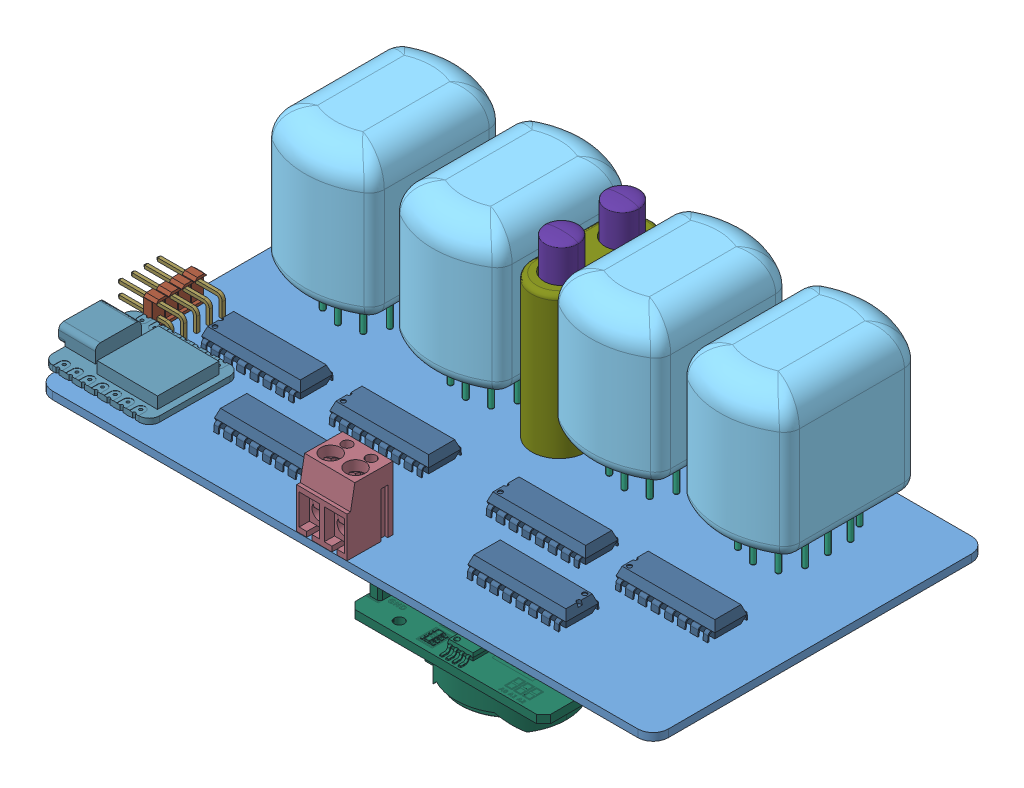
SolidWorks assembly nixie-display, configuration Défaut. Lengths in mm.
Overall size (127.16 50.53 67.27).
292 component instances, 54 part files, 24 mates.
Components (placement in the parent):
- pcb-1: pcb [Défaut] at origin size (121.6 1.5 65.9)
- IN-12A.stp-1: IN-12A.stp [Défaut] at (-40.9487 32.5 -15.5981) x (0 1 0) z (1 0 0) size (35 31 21)
  - 2.stp-1: 2.stp [Défaut] at origin size (2.7 24.17 15.83)
  - 3.stp-1: 3.stp [Défaut] at (-12.2 0 0) x (0 0 -1) z (-1 0 0) size (2 1.5 18.5)
  - 4.stp-1: 4.stp [Défaut] at (-12.2 0 0) x (0 0 1) z (-1 0 0) size (2 1.5 18.5)
  - 5.stp-1: 5.stp [Défaut] at (-12 0 0) x (0 0 -1) z (1 0 0) size (2.1 2.1 1)
  - 5.stp-2: 5.stp [Défaut] at (-10.8 0 0) x (0 0 -1) z (1 0 0) size (2.1 2.1 1)
  - 5.stp-3: 5.stp [Défaut] at (-9.6 0 0) x (0 0 -1) z (1 0 0) size (2.1 2.1 1)
  - 5.stp-4: 5.stp [Défaut] at (-8.4 0 0) x (0 0 -1) z (1 0 0) size (2.1 2.1 1)
  - 5.stp-5: 5.stp [Défaut] at (-7.2 0 0) x (0 0 -1) z (1 0 0) size (2.1 2.1 1)
  - 5.stp-6: 5.stp [Défaut] at (-6 0 0) x (0 0 -1) z (1 0 0) size (2.1 2.1 1)
  - 5.stp-7: 5.stp [Défaut] at (-4.8 0 0) x (0 0 -1) z (1 0 0) size (2.1 2.1 1)
  - 5.stp-8: 5.stp [Défaut] at (-3.6 0 0) x (0 0 -1) z (1 0 0) size (2.1 2.1 1)
  - 5.stp-9: 5.stp [Défaut] at (-2.4 0 0) x (0 0 -1) z (1 0 0) size (2.1 2.1 1)
  - 5.stp-10: 5.stp [Défaut] at (-1.2 0 0) x (0 0 -1) z (1 0 0) size (2.1 2.1 1)
  - 6.stp-1: 6.stp [Défaut] at (-11 16.1596 7.8778) x (0 -0.787778 0.61596) z (-1 0 0) size (2.1 2.1 1)
  - 7.stp-1: 7.stp [Défaut] at (-9.8 16.1596 7.8778) x (0 -0.787778 0.61596) z (-1 0 0) size (2.1 2.1 1)
  - 8.stp-1: 8.stp [Défaut] at (-8.6 16.1596 7.8778) x (0 -0.787778 0.61596) z (-1 0 0) size (2.1 2.1 1)
  - 9.stp-1: 9.stp [Défaut] at (-7.4 16.1596 7.8778) x (0 -0.787778 0.61596) z (-1 0 0) size (2.1 2.1 1)
  - 10.stp-1: 10.stp [Défaut] at (-6.2 16.1596 7.8778) x (0 -0.787778 0.61596) z (-1 0 0) size (2.1 2.1 1)
  - 11.stp-1: 11.stp [Défaut] at (-5 16.1596 7.8778) x (0 -0.787778 0.61596) z (-1 0 0) size (2.1 2.1 1)
  - 12.stp-1: 12.stp [Défaut] at (-3.8 16.1596 7.8778) x (0 -0.787778 0.61596) z (-1 0 0) size (2.1 2.1 1)
  - 13.stp-1: 13.stp [Défaut] at (-2.6 16.1596 7.8778) x (0 -0.787778 0.61596) z (-1 0 0) size (2.1 2.1 1)
  - 14.stp-1: 14.stp [Défaut] at (-1.4 16.1596 7.8778) x (0 -0.787778 0.61596) z (-1 0 0) size (2.1 2.1 1)
  - 15.stp-1: 15.stp [Défaut] at (-0.2 16.1596 7.8778) x (0 -0.787778 0.61596) z (-1 0 0) size (2.1 2.1 1)
  - 5.stp-11: 5.stp [Défaut] x (0 0 -1) z (1 0 0) size (2.1 2.1 1)
  - 5.stp-12: 5.stp [Défaut] at (-13.2 0 0) x (0 0 -1) z (1 0 0) size (2.1 2.1 1)
  - 16.stp-1: 16.stp [Défaut] at (1 16.1596 7.8778) x (0 -0.787778 0.61596) z (-1 0 0) size (2.1 2.1 1)
  - 17.stp-1: 17.stp [Défaut] at (-12.2 16.1596 7.8778) x (0 -0.787778 0.61596) z (-1 0 0) size (2.1 2.1 1)
  - 18.stp-1: 18.stp [Défaut] at (-13.2 0 0) x (0 0 -1) z (-1 0 0) size (15.83 24.17 12.28)
  - 19.stp-1: 19.stp [Défaut] x (1 0 0) z (0 1 0) size (1.51 1.46 20.68)
  - 20.stp-1: 20.stp [Défaut] at (1 0 0) size (4 22.27 2.42)
  - 21.stp-1: 21.stp [Défaut] at (-13.4 0 0) x (0 0 -1) z (-1 0 0) size (15.83 24.17 1)
  - 22.stp-1: 22.stp [Défaut] at (-14.4 0 0) x (0 0 -1) z (-1 0 0) size (15.83 27.29 2)
  - 23.stp-1: 23.stp [Défaut] x (0 0 -1) z (-1 0 0) size (21 31 33)
  - 24.stp-1: 24.stp [Défaut] x (0 0 -1) z (-1 0 0) size (1 1 15.5)
  - 24.stp-2: 24.stp [Défaut] at (0 -4.5 0) x (0 0 -1) z (-1 0 0) size (1 1 15.5)
  - 24.stp-3: 24.stp [Défaut] at (0 -8 -1.75) x (0 0 -1) z (-1 0 0) size (1 1 15.5)
  - 24.stp-4: 24.stp [Défaut] at (0 -9 -5.75) x (0 0 -1) z (-1 0 0) size (1 1 15.5)
  - 24.stp-5: 24.stp [Défaut] at (0 -8 -9.75) x (0 0 -1) z (-1 0 0) size (1 1 15.5)
  - 24.stp-6: 24.stp [Défaut] at (0 -4.5 -11.5) x (0 0 -1) z (-1 0 0) size (1 1 15.5)
  - 24.stp-7: 24.stp [Défaut] at (0 0 -11.5) x (0 0 -1) z (-1 0 0) size (1 1 15.5)
  - 24.stp-8: 24.stp [Défaut] at (0 4.5 -11.5) x (0 0 -1) z (-1 0 0) size (1 1 15.5)
  - 24.stp-9: 24.stp [Défaut] at (0 8 -9.75) x (0 0 -1) z (-1 0 0) size (1 1 15.5)
  - 24.stp-10: 24.stp [Défaut] at (0 9 -5.75) x (0 0 -1) z (-1 0 0) size (1 1 15.5)
  - 24.stp-11: 24.stp [Défaut] at (0 8 -1.75) x (0 0 -1) z (-1 0 0) size (1 1 15.5)
  - 24.stp-12: 24.stp [Défaut] at (0 4.5 0) x (0 0 -1) z (-1 0 0) size (1 1 15.5)
  - 25.stp-1: 25.stp [Défaut] at (-1.4 0 0) x (0 0 1) z (1 0 0) size (10.55 22 0.2)
  - 26.stp-1: 26.stp [Défaut] at (-2.6 0 0) x (0 0 1) z (1 0 0) size (11 22 0.2)
  - 27.stp-1: 27.stp [Défaut] at (-3.8 0 0) x (0 0 1) z (1 0 0) size (11 22 0.2)
  - 28.stp-1: 28.stp [Défaut] at (-5 0 0) x (0 0 1) z (1 0 0) size (10 22 0.2)
  - 29.stp-1: 29.stp [Défaut] at (-7.4 0 0) x (0 0 1) z (1 0 0) size (10 22 0.2)
  - 30.stp-1: 30.stp [Défaut] at (-9.6 0 0) x (0 0 -1) z (-1 0 0) size (10 22 0.2)
  - 31.stp-1: 31.stp [Défaut] at (-11 0 0) x (0 0 1) z (1 0 0) size (11 22 0.2)
  - 32.stp-1: 32.stp [Défaut] at (-12.2 0 0) x (0 0 1) z (1 0 0) size (2 22 0.2)
  - 33.stp-1: 33.stp [Défaut] at (-6 0 0) x (0 0 -1) z (-1 0 0) size (11 22 0.2)
  - 34.stp-1: 34.stp [Défaut] at (-8.6 0 0) x (0 0 1) z (1 0 0) size (10 22 0.2)
  - 1.stp-1: 1.stp [Défaut] at origin size (7.54 3.19 3.19)
  - 1-0.stp-1: 1-0.stp [Défaut] at origin size (11.99 9.11 6.32)
  - 1-1.stp-1: 1-1.stp [Défaut] at origin size (5.03 4.26 4.61)
  - 1-2.stp-1: 1-2.stp [Défaut] at origin size (8.17 8.42 6.65)
  - 1-3.stp-1: 1-3.stp [Défaut] at origin size (17.22 12.89 7.69)
  - 1-4.stp-1: 1-4.stp [Défaut] at origin size (13.11 12.81 7.39)
  - 1-5.stp-1: 1-5.stp [Défaut] at origin size (15.91 7.54 6.9)
  - 1-6.stp-1: 1-6.stp [Défaut] at origin size (10.39 4.47 4.23)
  - 1-7.stp-1: 1-7.stp [Défaut] at origin size (7.32 4.98 2.44)
  - 1-8.stp-1: 1-8.stp [Défaut] at origin size (10.29 4.36 5.63)
  - 1-9.stp-1: 1-9.stp [Défaut] at origin size (12.89 8.1 7.83)
- IN-12A.stp-2: IN-12A.stp [Défaut] at (15.5408 32.5 -15.6508) x (0 1 0) z (1 0 0) size (35 31 21)
  - 2.stp-1: 2.stp [Défaut] at origin size (2.7 24.17 15.83)
  - 3.stp-1: 3.stp [Défaut] at (-12.2 0 0) x (0 0 -1) z (-1 0 0) size (2 1.5 18.5)
  - 4.stp-1: 4.stp [Défaut] at (-12.2 0 0) x (0 0 1) z (-1 0 0) size (2 1.5 18.5)
  - 5.stp-1: 5.stp [Défaut] at (-12 0 0) x (0 0 -1) z (1 0 0) size (2.1 2.1 1)
  - 5.stp-2: 5.stp [Défaut] at (-10.8 0 0) x (0 0 -1) z (1 0 0) size (2.1 2.1 1)
  - 5.stp-3: 5.stp [Défaut] at (-9.6 0 0) x (0 0 -1) z (1 0 0) size (2.1 2.1 1)
  - 5.stp-4: 5.stp [Défaut] at (-8.4 0 0) x (0 0 -1) z (1 0 0) size (2.1 2.1 1)
  - 5.stp-5: 5.stp [Défaut] at (-7.2 0 0) x (0 0 -1) z (1 0 0) size (2.1 2.1 1)
  - 5.stp-6: 5.stp [Défaut] at (-6 0 0) x (0 0 -1) z (1 0 0) size (2.1 2.1 1)
  - 5.stp-7: 5.stp [Défaut] at (-4.8 0 0) x (0 0 -1) z (1 0 0) size (2.1 2.1 1)
  - 5.stp-8: 5.stp [Défaut] at (-3.6 0 0) x (0 0 -1) z (1 0 0) size (2.1 2.1 1)
  - 5.stp-9: 5.stp [Défaut] at (-2.4 0 0) x (0 0 -1) z (1 0 0) size (2.1 2.1 1)
  - 5.stp-10: 5.stp [Défaut] at (-1.2 0 0) x (0 0 -1) z (1 0 0) size (2.1 2.1 1)
  - 6.stp-1: 6.stp [Défaut] at (-11 16.1596 7.8778) x (0 -0.787778 0.61596) z (-1 0 0) size (2.1 2.1 1)
  - 7.stp-1: 7.stp [Défaut] at (-9.8 16.1596 7.8778) x (0 -0.787778 0.61596) z (-1 0 0) size (2.1 2.1 1)
  - 8.stp-1: 8.stp [Défaut] at (-8.6 16.1596 7.8778) x (0 -0.787778 0.61596) z (-1 0 0) size (2.1 2.1 1)
  - 9.stp-1: 9.stp [Défaut] at (-7.4 16.1596 7.8778) x (0 -0.787778 0.61596) z (-1 0 0) size (2.1 2.1 1)
  - 10.stp-1: 10.stp [Défaut] at (-6.2 16.1596 7.8778) x (0 -0.787778 0.61596) z (-1 0 0) size (2.1 2.1 1)
  - 11.stp-1: 11.stp [Défaut] at (-5 16.1596 7.8778) x (0 -0.787778 0.61596) z (-1 0 0) size (2.1 2.1 1)
  - 12.stp-1: 12.stp [Défaut] at (-3.8 16.1596 7.8778) x (0 -0.787778 0.61596) z (-1 0 0) size (2.1 2.1 1)
  - 13.stp-1: 13.stp [Défaut] at (-2.6 16.1596 7.8778) x (0 -0.787778 0.61596) z (-1 0 0) size (2.1 2.1 1)
  - 14.stp-1: 14.stp [Défaut] at (-1.4 16.1596 7.8778) x (0 -0.787778 0.61596) z (-1 0 0) size (2.1 2.1 1)
  - 15.stp-1: 15.stp [Défaut] at (-0.2 16.1596 7.8778) x (0 -0.787778 0.61596) z (-1 0 0) size (2.1 2.1 1)
  - 5.stp-11: 5.stp [Défaut] x (0 0 -1) z (1 0 0) size (2.1 2.1 1)
  - 5.stp-12: 5.stp [Défaut] at (-13.2 0 0) x (0 0 -1) z (1 0 0) size (2.1 2.1 1)
  - 16.stp-1: 16.stp [Défaut] at (1 16.1596 7.8778) x (0 -0.787778 0.61596) z (-1 0 0) size (2.1 2.1 1)
  - 17.stp-1: 17.stp [Défaut] at (-12.2 16.1596 7.8778) x (0 -0.787778 0.61596) z (-1 0 0) size (2.1 2.1 1)
  - 18.stp-1: 18.stp [Défaut] at (-13.2 0 0) x (0 0 -1) z (-1 0 0) size (15.83 24.17 12.28)
  - 19.stp-1: 19.stp [Défaut] x (1 0 0) z (0 1 0) size (1.51 1.46 20.68)
  - 20.stp-1: 20.stp [Défaut] at (1 0 0) size (4 22.27 2.42)
  - 21.stp-1: 21.stp [Défaut] at (-13.4 0 0) x (0 0 -1) z (-1 0 0) size (15.83 24.17 1)
  - 22.stp-1: 22.stp [Défaut] at (-14.4 0 0) x (0 0 -1) z (-1 0 0) size (15.83 27.29 2)
  - 23.stp-1: 23.stp [Défaut] x (0 0 -1) z (-1 0 0) size (21 31 33)
  - 24.stp-1: 24.stp [Défaut] x (0 0 -1) z (-1 0 0) size (1 1 15.5)
  - 24.stp-2: 24.stp [Défaut] at (0 -4.5 0) x (0 0 -1) z (-1 0 0) size (1 1 15.5)
  - 24.stp-3: 24.stp [Défaut] at (0 -8 -1.75) x (0 0 -1) z (-1 0 0) size (1 1 15.5)
  - 24.stp-4: 24.stp [Défaut] at (0 -9 -5.75) x (0 0 -1) z (-1 0 0) size (1 1 15.5)
  - 24.stp-5: 24.stp [Défaut] at (0 -8 -9.75) x (0 0 -1) z (-1 0 0) size (1 1 15.5)
  - 24.stp-6: 24.stp [Défaut] at (0 -4.5 -11.5) x (0 0 -1) z (-1 0 0) size (1 1 15.5)
  - 24.stp-7: 24.stp [Défaut] at (0 0 -11.5) x (0 0 -1) z (-1 0 0) size (1 1 15.5)
  - 24.stp-8: 24.stp [Défaut] at (0 4.5 -11.5) x (0 0 -1) z (-1 0 0) size (1 1 15.5)
  - 24.stp-9: 24.stp [Défaut] at (0 8 -9.75) x (0 0 -1) z (-1 0 0) size (1 1 15.5)
  - 24.stp-10: 24.stp [Défaut] at (0 9 -5.75) x (0 0 -1) z (-1 0 0) size (1 1 15.5)
  - 24.stp-11: 24.stp [Défaut] at (0 8 -1.75) x (0 0 -1) z (-1 0 0) size (1 1 15.5)
  - 24.stp-12: 24.stp [Défaut] at (0 4.5 0) x (0 0 -1) z (-1 0 0) size (1 1 15.5)
  - 25.stp-1: 25.stp [Défaut] at (-1.4 0 0) x (0 0 1) z (1 0 0) size (10.55 22 0.2)
  - 26.stp-1: 26.stp [Défaut] at (-2.6 0 0) x (0 0 1) z (1 0 0) size (11 22 0.2)
  - 27.stp-1: 27.stp [Défaut] at (-3.8 0 0) x (0 0 1) z (1 0 0) size (11 22 0.2)
  - 28.stp-1: 28.stp [Défaut] at (-5 0 0) x (0 0 1) z (1 0 0) size (10 22 0.2)
  - 29.stp-1: 29.stp [Défaut] at (-7.4 0 0) x (0 0 1) z (1 0 0) size (10 22 0.2)
  - 30.stp-1: 30.stp [Défaut] at (-9.6 0 0) x (0 0 -1) z (-1 0 0) size (10 22 0.2)
  - 31.stp-1: 31.stp [Défaut] at (-11 0 0) x (0 0 1) z (1 0 0) size (11 22 0.2)
  - 32.stp-1: 32.stp [Défaut] at (-12.2 0 0) x (0 0 1) z (1 0 0) size (2 22 0.2)
  - 33.stp-1: 33.stp [Défaut] at (-6 0 0) x (0 0 -1) z (-1 0 0) size (11 22 0.2)
  - 34.stp-1: 34.stp [Défaut] at (-8.6 0 0) x (0 0 1) z (1 0 0) size (10 22 0.2)
  - 1.stp-1: 1.stp [Défaut] at origin size (7.54 3.19 3.19)
  - 1-0.stp-1: 1-0.stp [Défaut] at origin size (11.99 9.11 6.32)
  - 1-1.stp-1: 1-1.stp [Défaut] at origin size (5.03 4.26 4.61)
  - 1-2.stp-1: 1-2.stp [Défaut] at origin size (8.17 8.42 6.65)
  - 1-3.stp-1: 1-3.stp [Défaut] at origin size (17.22 12.89 7.69)
  - 1-4.stp-1: 1-4.stp [Défaut] at origin size (13.11 12.81 7.39)
  - 1-5.stp-1: 1-5.stp [Défaut] at origin size (15.91 7.54 6.9)
  - 1-6.stp-1: 1-6.stp [Défaut] at origin size (10.39 4.47 4.23)
  - 1-7.stp-1: 1-7.stp [Défaut] at origin size (7.32 4.98 2.44)
  - 1-8.stp-1: 1-8.stp [Défaut] at origin size (10.29 4.36 5.63)
  - 1-9.stp-1: 1-9.stp [Défaut] at origin size (12.89 8.1 7.83)
- IN-12A.stp-3: IN-12A.stp [Défaut] at (-15.577 32.5 -15.4564) x (0 1 0) z (1 0 0) size (35 31 21)
  - 2.stp-1: 2.stp [Défaut] at origin size (2.7 24.17 15.83)
  - 3.stp-1: 3.stp [Défaut] at (-12.2 0 0) x (0 0 -1) z (-1 0 0) size (2 1.5 18.5)
  - 4.stp-1: 4.stp [Défaut] at (-12.2 0 0) x (0 0 1) z (-1 0 0) size (2 1.5 18.5)
  - 5.stp-1: 5.stp [Défaut] at (-12 0 0) x (0 0 -1) z (1 0 0) size (2.1 2.1 1)
  - 5.stp-2: 5.stp [Défaut] at (-10.8 0 0) x (0 0 -1) z (1 0 0) size (2.1 2.1 1)
  - 5.stp-3: 5.stp [Défaut] at (-9.6 0 0) x (0 0 -1) z (1 0 0) size (2.1 2.1 1)
  - 5.stp-4: 5.stp [Défaut] at (-8.4 0 0) x (0 0 -1) z (1 0 0) size (2.1 2.1 1)
  - 5.stp-5: 5.stp [Défaut] at (-7.2 0 0) x (0 0 -1) z (1 0 0) size (2.1 2.1 1)
  - 5.stp-6: 5.stp [Défaut] at (-6 0 0) x (0 0 -1) z (1 0 0) size (2.1 2.1 1)
  - 5.stp-7: 5.stp [Défaut] at (-4.8 0 0) x (0 0 -1) z (1 0 0) size (2.1 2.1 1)
  - 5.stp-8: 5.stp [Défaut] at (-3.6 0 0) x (0 0 -1) z (1 0 0) size (2.1 2.1 1)
  - 5.stp-9: 5.stp [Défaut] at (-2.4 0 0) x (0 0 -1) z (1 0 0) size (2.1 2.1 1)
  - 5.stp-10: 5.stp [Défaut] at (-1.2 0 0) x (0 0 -1) z (1 0 0) size (2.1 2.1 1)
  - 6.stp-1: 6.stp [Défaut] at (-11 16.1596 7.8778) x (0 -0.787778 0.61596) z (-1 0 0) size (2.1 2.1 1)
  - 7.stp-1: 7.stp [Défaut] at (-9.8 16.1596 7.8778) x (0 -0.787778 0.61596) z (-1 0 0) size (2.1 2.1 1)
  - 8.stp-1: 8.stp [Défaut] at (-8.6 16.1596 7.8778) x (0 -0.787778 0.61596) z (-1 0 0) size (2.1 2.1 1)
  - 9.stp-1: 9.stp [Défaut] at (-7.4 16.1596 7.8778) x (0 -0.787778 0.61596) z (-1 0 0) size (2.1 2.1 1)
  - 10.stp-1: 10.stp [Défaut] at (-6.2 16.1596 7.8778) x (0 -0.787778 0.61596) z (-1 0 0) size (2.1 2.1 1)
  - 11.stp-1: 11.stp [Défaut] at (-5 16.1596 7.8778) x (0 -0.787778 0.61596) z (-1 0 0) size (2.1 2.1 1)
  - 12.stp-1: 12.stp [Défaut] at (-3.8 16.1596 7.8778) x (0 -0.787778 0.61596) z (-1 0 0) size (2.1 2.1 1)
  - 13.stp-1: 13.stp [Défaut] at (-2.6 16.1596 7.8778) x (0 -0.787778 0.61596) z (-1 0 0) size (2.1 2.1 1)
  - 14.stp-1: 14.stp [Défaut] at (-1.4 16.1596 7.8778) x (0 -0.787778 0.61596) z (-1 0 0) size (2.1 2.1 1)
  - 15.stp-1: 15.stp [Défaut] at (-0.2 16.1596 7.8778) x (0 -0.787778 0.61596) z (-1 0 0) size (2.1 2.1 1)
  - 5.stp-11: 5.stp [Défaut] x (0 0 -1) z (1 0 0) size (2.1 2.1 1)
  - 5.stp-12: 5.stp [Défaut] at (-13.2 0 0) x (0 0 -1) z (1 0 0) size (2.1 2.1 1)
  - 16.stp-1: 16.stp [Défaut] at (1 16.1596 7.8778) x (0 -0.787778 0.61596) z (-1 0 0) size (2.1 2.1 1)
  - 17.stp-1: 17.stp [Défaut] at (-12.2 16.1596 7.8778) x (0 -0.787778 0.61596) z (-1 0 0) size (2.1 2.1 1)
  - 18.stp-1: 18.stp [Défaut] at (-13.2 0 0) x (0 0 -1) z (-1 0 0) size (15.83 24.17 12.28)
  - 19.stp-1: 19.stp [Défaut] x (1 0 0) z (0 1 0) size (1.51 1.46 20.68)
  - 20.stp-1: 20.stp [Défaut] at (1 0 0) size (4 22.27 2.42)
  - 21.stp-1: 21.stp [Défaut] at (-13.4 0 0) x (0 0 -1) z (-1 0 0) size (15.83 24.17 1)
  - 22.stp-1: 22.stp [Défaut] at (-14.4 0 0) x (0 0 -1) z (-1 0 0) size (15.83 27.29 2)
  - 23.stp-1: 23.stp [Défaut] x (0 0 -1) z (-1 0 0) size (21 31 33)
  - 24.stp-1: 24.stp [Défaut] x (0 0 -1) z (-1 0 0) size (1 1 15.5)
  - 24.stp-2: 24.stp [Défaut] at (0 -4.5 0) x (0 0 -1) z (-1 0 0) size (1 1 15.5)
  - 24.stp-3: 24.stp [Défaut] at (0 -8 -1.75) x (0 0 -1) z (-1 0 0) size (1 1 15.5)
  - 24.stp-4: 24.stp [Défaut] at (0 -9 -5.75) x (0 0 -1) z (-1 0 0) size (1 1 15.5)
  - 24.stp-5: 24.stp [Défaut] at (0 -8 -9.75) x (0 0 -1) z (-1 0 0) size (1 1 15.5)
  - 24.stp-6: 24.stp [Défaut] at (0 -4.5 -11.5) x (0 0 -1) z (-1 0 0) size (1 1 15.5)
  - 24.stp-7: 24.stp [Défaut] at (0 0 -11.5) x (0 0 -1) z (-1 0 0) size (1 1 15.5)
  - 24.stp-8: 24.stp [Défaut] at (0 4.5 -11.5) x (0 0 -1) z (-1 0 0) size (1 1 15.5)
  - 24.stp-9: 24.stp [Défaut] at (0 8 -9.75) x (0 0 -1) z (-1 0 0) size (1 1 15.5)
  - 24.stp-10: 24.stp [Défaut] at (0 9 -5.75) x (0 0 -1) z (-1 0 0) size (1 1 15.5)
  - 24.stp-11: 24.stp [Défaut] at (0 8 -1.75) x (0 0 -1) z (-1 0 0) size (1 1 15.5)
  - 24.stp-12: 24.stp [Défaut] at (0 4.5 0) x (0 0 -1) z (-1 0 0) size (1 1 15.5)
  - 25.stp-1: 25.stp [Défaut] at (-1.4 0 0) x (0 0 1) z (1 0 0) size (10.55 22 0.2)
  - 26.stp-1: 26.stp [Défaut] at (-2.6 0 0) x (0 0 1) z (1 0 0) size (11 22 0.2)
  - 27.stp-1: 27.stp [Défaut] at (-3.8 0 0) x (0 0 1) z (1 0 0) size (11 22 0.2)
  - 28.stp-1: 28.stp [Défaut] at (-5 0 0) x (0 0 1) z (1 0 0) size (10 22 0.2)
  - 29.stp-1: 29.stp [Défaut] at (-7.4 0 0) x (0 0 1) z (1 0 0) size (10 22 0.2)
  - 30.stp-1: 30.stp [Défaut] at (-9.6 0 0) x (0 0 -1) z (-1 0 0) size (10 22 0.2)
  - 31.stp-1: 31.stp [Défaut] at (-11 0 0) x (0 0 1) z (1 0 0) size (11 22 0.2)
  - 32.stp-1: 32.stp [Défaut] at (-12.2 0 0) x (0 0 1) z (1 0 0) size (2 22 0.2)
  - 33.stp-1: 33.stp [Défaut] at (-6 0 0) x (0 0 -1) z (-1 0 0) size (11 22 0.2)
  - 34.stp-1: 34.stp [Défaut] at (-8.6 0 0) x (0 0 1) z (1 0 0) size (10 22 0.2)
  - 1.stp-1: 1.stp [Défaut] at origin size (7.54 3.19 3.19)
  - 1-0.stp-1: 1-0.stp [Défaut] at origin size (11.99 9.11 6.32)
  - 1-1.stp-1: 1-1.stp [Défaut] at origin size (5.03 4.26 4.61)
  - 1-2.stp-1: 1-2.stp [Défaut] at origin size (8.17 8.42 6.65)
  - 1-3.stp-1: 1-3.stp [Défaut] at origin size (17.22 12.89 7.69)
  - 1-4.stp-1: 1-4.stp [Défaut] at origin size (13.11 12.81 7.39)
  - 1-5.stp-1: 1-5.stp [Défaut] at origin size (15.91 7.54 6.9)
  - 1-6.stp-1: 1-6.stp [Défaut] at origin size (10.39 4.47 4.23)
  - 1-7.stp-1: 1-7.stp [Défaut] at origin size (7.32 4.98 2.44)
  - 1-8.stp-1: 1-8.stp [Défaut] at origin size (10.29 4.36 5.63)
  - 1-9.stp-1: 1-9.stp [Défaut] at origin size (12.89 8.1 7.83)
- IN-12A.stp-4: IN-12A.stp [Défaut] at (40.934 32.5 -15.666) x (0 1 0) z (1 0 0) size (35 31 21)
  - 2.stp-1: 2.stp [Défaut] at origin size (2.7 24.17 15.83)
  - 3.stp-1: 3.stp [Défaut] at (-12.2 0 0) x (0 0 -1) z (-1 0 0) size (2 1.5 18.5)
  - 4.stp-1: 4.stp [Défaut] at (-12.2 0 0) x (0 0 1) z (-1 0 0) size (2 1.5 18.5)
  - 5.stp-1: 5.stp [Défaut] at (-12 0 0) x (0 0 -1) z (1 0 0) size (2.1 2.1 1)
  - 5.stp-2: 5.stp [Défaut] at (-10.8 0 0) x (0 0 -1) z (1 0 0) size (2.1 2.1 1)
  - 5.stp-3: 5.stp [Défaut] at (-9.6 0 0) x (0 0 -1) z (1 0 0) size (2.1 2.1 1)
  - 5.stp-4: 5.stp [Défaut] at (-8.4 0 0) x (0 0 -1) z (1 0 0) size (2.1 2.1 1)
  - 5.stp-5: 5.stp [Défaut] at (-7.2 0 0) x (0 0 -1) z (1 0 0) size (2.1 2.1 1)
  - 5.stp-6: 5.stp [Défaut] at (-6 0 0) x (0 0 -1) z (1 0 0) size (2.1 2.1 1)
  - 5.stp-7: 5.stp [Défaut] at (-4.8 0 0) x (0 0 -1) z (1 0 0) size (2.1 2.1 1)
  - 5.stp-8: 5.stp [Défaut] at (-3.6 0 0) x (0 0 -1) z (1 0 0) size (2.1 2.1 1)
  - 5.stp-9: 5.stp [Défaut] at (-2.4 0 0) x (0 0 -1) z (1 0 0) size (2.1 2.1 1)
  - 5.stp-10: 5.stp [Défaut] at (-1.2 0 0) x (0 0 -1) z (1 0 0) size (2.1 2.1 1)
  - 6.stp-1: 6.stp [Défaut] at (-11 16.1596 7.8778) x (0 -0.787778 0.61596) z (-1 0 0) size (2.1 2.1 1)
  - 7.stp-1: 7.stp [Défaut] at (-9.8 16.1596 7.8778) x (0 -0.787778 0.61596) z (-1 0 0) size (2.1 2.1 1)
  - 8.stp-1: 8.stp [Défaut] at (-8.6 16.1596 7.8778) x (0 -0.787778 0.61596) z (-1 0 0) size (2.1 2.1 1)
  - 9.stp-1: 9.stp [Défaut] at (-7.4 16.1596 7.8778) x (0 -0.787778 0.61596) z (-1 0 0) size (2.1 2.1 1)
  - 10.stp-1: 10.stp [Défaut] at (-6.2 16.1596 7.8778) x (0 -0.787778 0.61596) z (-1 0 0) size (2.1 2.1 1)
  - 11.stp-1: 11.stp [Défaut] at (-5 16.1596 7.8778) x (0 -0.787778 0.61596) z (-1 0 0) size (2.1 2.1 1)
  - 12.stp-1: 12.stp [Défaut] at (-3.8 16.1596 7.8778) x (0 -0.787778 0.61596) z (-1 0 0) size (2.1 2.1 1)
  - 13.stp-1: 13.stp [Défaut] at (-2.6 16.1596 7.8778) x (0 -0.787778 0.61596) z (-1 0 0) size (2.1 2.1 1)
  - 14.stp-1: 14.stp [Défaut] at (-1.4 16.1596 7.8778) x (0 -0.787778 0.61596) z (-1 0 0) size (2.1 2.1 1)
  - 15.stp-1: 15.stp [Défaut] at (-0.2 16.1596 7.8778) x (0 -0.787778 0.61596) z (-1 0 0) size (2.1 2.1 1)
  - 5.stp-11: 5.stp [Défaut] x (0 0 -1) z (1 0 0) size (2.1 2.1 1)
  - 5.stp-12: 5.stp [Défaut] at (-13.2 0 0) x (0 0 -1) z (1 0 0) size (2.1 2.1 1)
  - 16.stp-1: 16.stp [Défaut] at (1 16.1596 7.8778) x (0 -0.787778 0.61596) z (-1 0 0) size (2.1 2.1 1)
  - 17.stp-1: 17.stp [Défaut] at (-12.2 16.1596 7.8778) x (0 -0.787778 0.61596) z (-1 0 0) size (2.1 2.1 1)
  - 18.stp-1: 18.stp [Défaut] at (-13.2 0 0) x (0 0 -1) z (-1 0 0) size (15.83 24.17 12.28)
  - 19.stp-1: 19.stp [Défaut] x (1 0 0) z (0 1 0) size (1.51 1.46 20.68)
  - 20.stp-1: 20.stp [Défaut] at (1 0 0) size (4 22.27 2.42)
  - 21.stp-1: 21.stp [Défaut] at (-13.4 0 0) x (0 0 -1) z (-1 0 0) size (15.83 24.17 1)
  - 22.stp-1: 22.stp [Défaut] at (-14.4 0 0) x (0 0 -1) z (-1 0 0) size (15.83 27.29 2)
  - 23.stp-1: 23.stp [Défaut] x (0 0 -1) z (-1 0 0) size (21 31 33)
  - 24.stp-1: 24.stp [Défaut] x (0 0 -1) z (-1 0 0) size (1 1 15.5)
  - 24.stp-2: 24.stp [Défaut] at (0 -4.5 0) x (0 0 -1) z (-1 0 0) size (1 1 15.5)
  - 24.stp-3: 24.stp [Défaut] at (0 -8 -1.75) x (0 0 -1) z (-1 0 0) size (1 1 15.5)
  - 24.stp-4: 24.stp [Défaut] at (0 -9 -5.75) x (0 0 -1) z (-1 0 0) size (1 1 15.5)
  - 24.stp-5: 24.stp [Défaut] at (0 -8 -9.75) x (0 0 -1) z (-1 0 0) size (1 1 15.5)
  - 24.stp-6: 24.stp [Défaut] at (0 -4.5 -11.5) x (0 0 -1) z (-1 0 0) size (1 1 15.5)
  - 24.stp-7: 24.stp [Défaut] at (0 0 -11.5) x (0 0 -1) z (-1 0 0) size (1 1 15.5)
  - 24.stp-8: 24.stp [Défaut] at (0 4.5 -11.5) x (0 0 -1) z (-1 0 0) size (1 1 15.5)
  - 24.stp-9: 24.stp [Défaut] at (0 8 -9.75) x (0 0 -1) z (-1 0 0) size (1 1 15.5)
  - 24.stp-10: 24.stp [Défaut] at (0 9 -5.75) x (0 0 -1) z (-1 0 0) size (1 1 15.5)
  - 24.stp-11: 24.stp [Défaut] at (0 8 -1.75) x (0 0 -1) z (-1 0 0) size (1 1 15.5)
  - 24.stp-12: 24.stp [Défaut] at (0 4.5 0) x (0 0 -1) z (-1 0 0) size (1 1 15.5)
  - 25.stp-1: 25.stp [Défaut] at (-1.4 0 0) x (0 0 1) z (1 0 0) size (10.55 22 0.2)
  - 26.stp-1: 26.stp [Défaut] at (-2.6 0 0) x (0 0 1) z (1 0 0) size (11 22 0.2)
  - 27.stp-1: 27.stp [Défaut] at (-3.8 0 0) x (0 0 1) z (1 0 0) size (11 22 0.2)
  - 28.stp-1: 28.stp [Défaut] at (-5 0 0) x (0 0 1) z (1 0 0) size (10 22 0.2)
  - 29.stp-1: 29.stp [Défaut] at (-7.4 0 0) x (0 0 1) z (1 0 0) size (10 22 0.2)
  - 30.stp-1: 30.stp [Défaut] at (-9.6 0 0) x (0 0 -1) z (-1 0 0) size (10 22 0.2)
  - 31.stp-1: 31.stp [Défaut] at (-11 0 0) x (0 0 1) z (1 0 0) size (11 22 0.2)
  - 32.stp-1: 32.stp [Défaut] at (-12.2 0 0) x (0 0 1) z (1 0 0) size (2 22 0.2)
  - 33.stp-1: 33.stp [Défaut] at (-6 0 0) x (0 0 -1) z (-1 0 0) size (11 22 0.2)
  - 34.stp-1: 34.stp [Défaut] at (-8.6 0 0) x (0 0 1) z (1 0 0) size (10 22 0.2)
  - 1.stp-1: 1.stp [Défaut] at origin size (7.54 3.19 3.19)
  - 1-0.stp-1: 1-0.stp [Défaut] at origin size (11.99 9.11 6.32)
  - 1-1.stp-1: 1-1.stp [Défaut] at origin size (5.03 4.26 4.61)
  - 1-2.stp-1: 1-2.stp [Défaut] at origin size (8.17 8.42 6.65)
  - 1-3.stp-1: 1-3.stp [Défaut] at origin size (17.22 12.89 7.69)
  - 1-4.stp-1: 1-4.stp [Défaut] at origin size (13.11 12.81 7.39)
  - 1-5.stp-1: 1-5.stp [Défaut] at origin size (15.91 7.54 6.9)
  - 1-6.stp-1: 1-6.stp [Défaut] at origin size (10.39 4.47 4.23)
  - 1-7.stp-1: 1-7.stp [Défaut] at origin size (7.32 4.98 2.44)
  - 1-8.stp-1: 1-8.stp [Défaut] at origin size (10.29 4.36 5.63)
  - 1-9.stp-1: 1-9.stp [Défaut] at origin size (12.89 8.1 7.83)
- DIP18N.step-1: DIP18N.step [Défaut] at (-50.7835 3.7087 35.4382) x (0 0 1) z (-1 0 0) size (8.53 6.85 19.5)
- DIP18N.step-2: DIP18N.step [Défaut] at (31.1067 3.7087 35.4997) x (0 0 1) z (-1 0 0) size (8.53 6.85 19.5)
- DIP18N.step-3: DIP18N.step [Défaut] at (5.6608 3.7087 35.5611) x (0 0 1) z (-1 0 0) size (8.53 6.85 19.5)
- DIP18N.step-4: DIP18N.step [Défaut] at (-25.3559 3.7087 35.5399) x (0 0 1) z (-1 0 0) size (8.53 6.85 19.5)
- DS1022-2x4RF11.stp-1: DS1022-2x4RF11.stp [Défaut] at (-56.1796 1.5 3.5604) x (0 0 1) z (0 1 0) size (10.16 13.04 8)
  - eBom-prt0.stp-1: eBom-prt0.stp [Défaut] at origin size (10.16 2.5 5)
  - eBom-prt1.stp-1: eBom-prt1.stp [Défaut] at origin size (0.64 13.04 7.09)
  - eBom-prt1.stp-2: eBom-prt1.stp [Défaut] at (2.54 0 0) size (0.64 13.04 7.09)
  - eBom-prt1.stp-3: eBom-prt1.stp [Défaut] at (5.08 0 0) size (0.64 13.04 7.09)
  - eBom-prt1.stp-4: eBom-prt1.stp [Défaut] at (7.62 0 0) size (0.64 13.04 7.09)
- DIP18N.step-5: DIP18N.step [Défaut] at (-15.751 3.7087 -7.8923) x (0.008727 0 -0.999962) z (0.999962 0 0.008727) size (8.53 6.85 19.5)
- DIP18N.step-6: DIP18N.step [Défaut] at (34.3108 3.7087 -7.8662) x (0.008727 0 -0.999962) z (0.999962 0 0.008727) size (8.53 6.85 19.5)
- Screw Terminal Block 5mm-2: Screw Terminal Block 5mm [Valor predeterminado] at (0.4217 1.5 23.933) x (-0.999962 0 -0.008727) z (0.008727 0 -0.999962) size (10.6 16.9 9)
- Seeeduino Xiao.step-1: Seeeduino Xiao.step [Défaut] at (-88.5187 11.44 25.9289) x (-0.008727 0 0.999962) z (-0.999962 0 -0.008727) size (17.8 4.27 22.5)
- DS3231 RTC.step-1: DS3231 RTC.step [Défaut] at (21.2627 -4.62 22.922) x (1 0 0) z (0 1 0) size (44.75 22.8 13.53)
- indics-1: indics [Défaut] at (0 1.5 -21.8057) size (10.8 43.17 23.8)
  - indic-holder-1: indic-holder [Défaut] at (0 0 6) size (10.8 28.02 23.8)
  - INS1.STEP-1: INS1.STEP [Défaut] at (0 17 0) x (0 0 1) z (-1 0 0) size (7.01 43.17 6.51)
    - INS1-Glask_rper_01.STEP-1: INS1-Glask_rper_01.STEP [Défaut] at origin size (7.01 28.6 6.51)
    - INS1_Inlay_01.STEP-1: INS1_Inlay_01.STEP [Défaut] at (0 5.1 0) size (6 41.77 5.25)
  - INS1.STEP-2: INS1.STEP [Défaut] at (0 17 12) x (0 0 1) z (-1 0 0) size (7.01 43.17 6.51)
    - INS1-Glask_rper_01.STEP-1: INS1-Glask_rper_01.STEP [Défaut] at origin size (7.01 28.6 6.51)
    - INS1_Inlay_01.STEP-1: INS1_Inlay_01.STEP [Défaut] at (0 5.1 0) size (6 41.77 5.25)
Mates (geometry in assembly coordinates):
- Coïncidente5: coincident anti-aligned: plane of pcb-1 through (0 1.5 0) normal (0 1 0); plane of IN-12A.stp-1/24.stp-8 through (-52.4487 1.5 -11.0981) normal (0 -1 0)
- Parallèle3: parallel aligned: plane of pcb-1 through (-60.8 1.5 -32.95) normal (-1 0 0); plane of IN-12A.stp-1/23.stp-1 through (-51.4487 36.5 -5.24) normal (-1 0 0)
- Coïncidente7: coincident anti-aligned: plane of pcb-1 through (0 1.5 0) normal (0 1 0); plane of IN-12A.stp-3/24.stp-2 through (-15.577 1.5 -19.9564) normal (0 -1 0)
- Coïncidente9: coincident anti-aligned: plane of pcb-1 through (0 1.5 0) normal (0 1 0); plane of IN-12A.stp-4/24.stp-10 through (35.184 1.5 -6.666) normal (0 -1 0)
- Parallèle5: parallel aligned: plane of IN-12A.stp-1/23.stp-1 through (-51.4487 36.5 -5.24) normal (-1 0 0); plane of IN-12A.stp-4/23.stp-1 through (30.434 36.5 -5.308) normal (-1 0 0)
- Coïncidente11: coincident anti-aligned: plane of pcb-1 through (0 1.5 0) normal (0 1 0); circle of IN-12A.stp-2/24.stp-6
- Parallèle6: parallel aligned: plane of IN-12A.stp-1/23.stp-1 through (-51.4487 36.5 -5.24) normal (-1 0 0); plane of IN-12A.stp-2/23.stp-1 through (5.0408 36.5 -5.2927) normal (-1 0 0)
- Coïncidente15: coincident anti-aligned: plane of pcb-1 through (0 1.5 0) normal (0 1 0); plane of DIP18N.step-1 through (-31.2835 1.5 4.7548) normal (0 -1 0)
- Coïncidente16: coincident anti-aligned: plane of pcb-1 through (0 1.5 0) normal (0 1 0); plane of DIP18N.step-4 through (-5.8559 1.5 4.8565) normal (0 -1 0)
- Coïncidente17: coincident anti-aligned: plane of pcb-1 through (0 1.5 0) normal (0 1 0); plane of DIP18N.step-3 through (25.1608 1.5 4.8776) normal (0 -1 0)
- Coïncidente18: coincident anti-aligned: plane of pcb-1 through (0 1.5 0) normal (0 1 0); plane of DIP18N.step-2 through (50.6067 1.5 4.8163) normal (0 -1 0)
- Coïncidente19: coincident anti-aligned: plane of pcb-1 through (0 1.5 0) normal (0 1 0); plane of DS1022-2x4RF11.stp-1/eBom-prt0.stp-1 through (-60.3596 1.5 4.2457) normal (0 -1 0)
- Parallèle7: parallel aligned: plane of pcb-1 through (-60.8 1.5 -32.95) normal (-1 0 0); plane of DS1022-2x4RF11.stp-1/eBom-prt0.stp-1 through (-60.3596 1.5 3.5604) normal (-1 0 0)
- Coïncidente21: coincident anti-aligned: plane of pcb-1 through (0 1.5 0) normal (0 1 0); plane of DIP18N.step-5 through (-35.5181 1.5 22.6198) normal (0 -1 0)
- Coïncidente22: coincident anti-aligned: plane of pcb-1 through (0 1.5 0) normal (0 1 0); plane of DIP18N.step-6 through (14.5438 1.5 22.6458) normal (0 -1 0)
- Coïncidente23: coincident anti-aligned: plane of pcb-1 through (0 1.5 0) normal (0 1 0); plane of Screw Terminal Block 5mm-2 through (-9.6565 1.5 32.8454) normal (0 -1 0)
- Distance1: distance = 2.5 mm anti-aligned: plane of Seeeduino Xiao.step-1 through (-49.894 4 23.2659) normal (0 -1 0); plane of pcb-1 through (0 1.5 0) normal (0 1 0)
- Coïncidente26: coincident aligned: plane of pcb-1 through (0 0 0) normal (1 0 0)
- Coïncidente27: coincident aligned: plane of pcb-1 through (0 0 0) normal (0 0 1)
- Coïncidente28: coincident aligned: plane of pcb-1 through (0 0 0) normal (0 1 0)
- Parallèle8: parallel anti-aligned: plane of pcb-1 through (0 0 0) normal (0 -1 0); plane of DS3231 RTC.step-1 through (21.2627 -4.62 22.922) normal (0 1 0)
- Distance2: distance = 4.62 mm anti-aligned: plane of pcb-1 through (0 0 0) normal (0 -1 0); plane of DS3231 RTC.step-1 through (21.2627 -4.62 22.922) normal (0 1 0)
- Coïncidente29: coincident anti-aligned: plane of pcb-1 through (0 1.5 0) normal (0 1 0); plane of indics-1/indic-holder-1 through (0 1.5 -22.3057) normal (0 -1 0)
- Coïncidente30: coincident aligned: plane of indics-1 through (0 1.5 -21.8057) normal (1 0 0)
